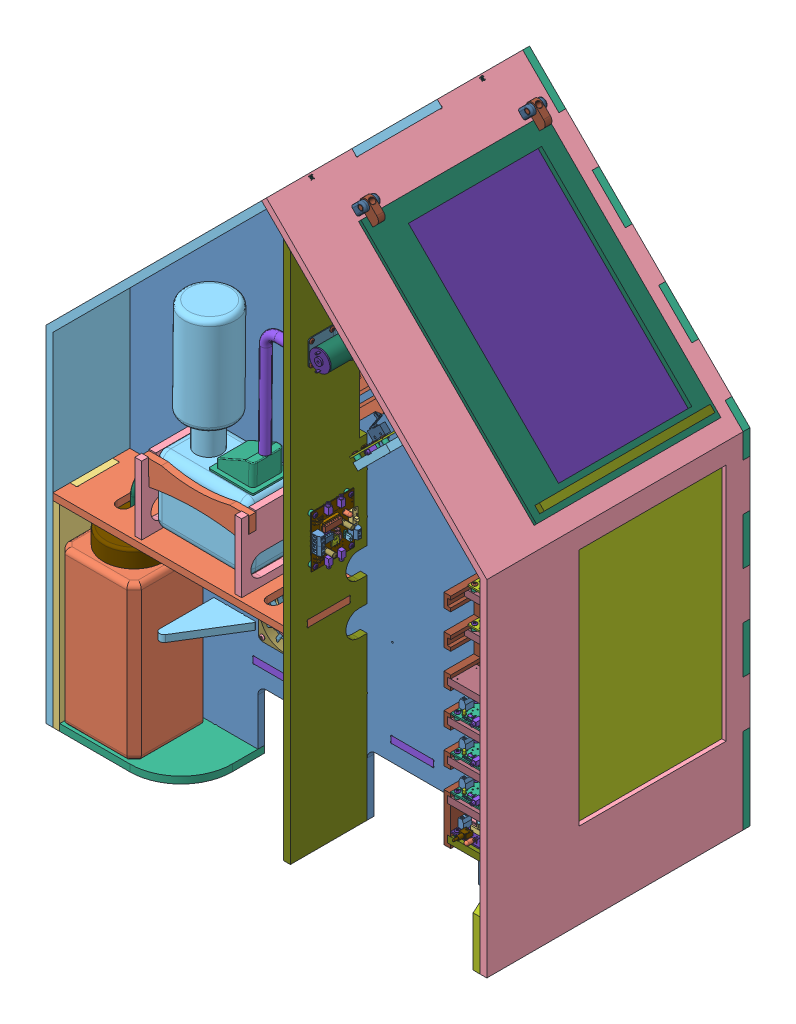
SolidWorks assembly Serre Toutes Options, configuration OLED. Lengths in mm. (continued)
Components (placement in the parent): (continued)
- VIS TORCX TF 3 X 19-50: VIS TORCX TF 3 X 19 [Défaut] at (178.8547 -145.9656 -4) x (-0.923728 -0.383049 0) z (0 0 -1)
- VIS TORCX TF 3 X 19-51: VIS TORCX TF 3 X 19 [Défaut] at (116.8547 -145.9656 -4) x (-0.923728 -0.383049 0) z (0 0 -1)
- VIS TORCX TF 3 X 19-52: VIS TORCX TF 3 X 19 [Défaut] at (178.8547 -7.9656 -4) x (-0.923728 -0.383049 0) z (0 0 -1)
- VIS TORCX TF 3 X 19-53: VIS TORCX TF 3 X 19 [Défaut] at (116.8547 -7.9656 -4) x (-0.923728 -0.383049 0) z (0 0 -1)
- Sous ensemble Arrosage-1: Sous ensemble Arrosage [Défaut] at (-248.1801 -261.6655 37.8651) x (-0.00308 0 0.999995) z (0 -1 0) size (140.54 240.54 274.35)
  - Pompe-1: Pompe [Défaut] at (-9.0938 -0.5877 17.5) size (40 29 55)
  - Tuyau gouteur-1: Tuyau gouteur [Défaut] at (-69.6171 -162.8404 -195.5) x (0 0 -1) z (0.999995 -0.00308 0) size (203 173 86)
  - Gouteur-1: Gouteur [Défaut] at (-70.8858 -170.9803 -151.85) x (-0.999995 0.00308 0) z (0 0 1) size (21 26.3 133.2)
    - PiedGouteur-1: PiedGouteur [Défaut] at (-1.2437 2.6563 -65) size (16 23.8 130)
    - BouchonGouteur-1: BouchonGouteur [Défaut] at (-1.2437 2.6563 -57) x (-0.923728 -0.383049 0) z (0 0 -1) size (16.07 16.07 11.2)
  - Bouchon reservoir-1: Bouchon reservoir [Défaut] at (10.9062 6.9123 -125.7) x (0.574699 -0.818365 0) z (0.818365 0.574699 0) size (71 20 71)
  - Passe cable-1: Passe cable [Défaut] at (10.9062 6.9123 -169.9434) x (0 0 -1) z (0 1 0) size (6 11 11)
  - Reservoir 1,25L-1: Reservoir 1,25L [Défaut] at (7.3532 24.2973 -125.7) x (0.999995 -0.00308 0) z (0 0 1) size (89.5 89.5 187)
- fondcuivré-1: fondcuivré [Défaut] at (-208.3657 -251.1382 -5)
- Capot complet-1: Capot complet [Vitres] at (-187.0166 -15.8593 -60) x (-1 0 0) z (0 0 -1) size (516 661.85 308)
  - Capot coté droit-1: Capot coté droit [Défaut] at (-332.1697 -265.6526 -154) size (263.66 661.85 308)
  - Capot coté gauche-1: Capot coté gauche [Défaut] at (175.8303 -266.1888 -154) size (263.66 661.85 308)
  - Capotfaçade-1: Capotfaçade [Défaut] at (75.9652 -264.3201 154) x (-1 0 0) z (0 0 -1) size (516 661.85 8)
  - Vitre laterale-1: Vitre laterale [Défaut] at (-385.1406 -165.6883 102.4285) x (0 1 0) z (1 0 0) size (290.43 181.9 2)
  - Vitre avant grande-1: Vitre avant grande [Défaut] at (-355.6546 -169.3327 147) x (0 1 0) z (0 0 1) size (286.8 171.11 2)
  - Vitre laterale-2: Vitre laterale [Défaut] at (120.8594 30.4421 102.4285) x (0 -1 0) z (-1 0 0) size (290.43 181.9 2)
  - Vitre avant grande-2: Vitre avant grande [Défaut] at (-40.8684 -169.3327 147) x (0 1 0) z (0 0 1) size (286.8 171.11 2)
  - Vitre avant centrale-1: Vitre avant centrale [Défaut] at (-154.2178 43.2096 147) size (123.47 286.8 2)
  - Vitre laterale-4: Vitre laterale [Défaut] at (-65.085 276.7887 -22.3285) x (0.707107 -0.707107 0) z (0.707107 0.707107 0) size (290.43 181.9 2)
  - Charnière percée-1: Charnière percée [Défaut] at (-176.8635 321.0541 -74.2825) x (-0.707107 -0.707107 0) z (0 0 -1) size (25.5 17 19)
    - Charnière percée-1: Charnière percée [Défaut] at (-8.739 -12.0088 -9.5) size (11 16 19)
    - Charnièere percée  2-1: Charnièere percée  2 [Défaut] at (-8.739 1.9912 -4) size (25.5 13 19)
  - Charnière percée-2: Charnière percée [Défaut] at (-176.8635 321.0541 120.9123) x (-0.707107 -0.707107 0) z (0 0 -1) size (25.5 17 19)
    - Charnière percée-1: Charnière percée [Défaut] at (-8.739 -12.0088 -9.5) size (11 16 19)
    - Charnièere percée  2-1: Charnièere percée  2 [Défaut] at (-8.739 1.9912 -4) size (25.5 13 19)
  - VIS TORCX TF 3 X 13-4: VIS TORCX TF 3 X 13 [Défaut] at (-159.0106 315.56 -74.2825) x (0.5 0.5 -0.707107) z (0.707107 -0.707107 0) size (5.6 5.6 13)
  - VIS TORCX TF 3 X 13-5: VIS TORCX TF 3 X 13 [Défaut] at (-159.0106 315.56 120.9123) x (0.5 0.5 -0.707107) z (0.707107 -0.707107 0) size (5.6 5.6 13)
  - VIS TORCX TF 3 X 19-1: VIS TORCX TF 3 X 19 [Défaut] at (-386.1406 -283.1062 154)
  - VIS TORCX TF 3 X 19-2: VIS TORCX TF 3 X 19 [Défaut] at (-386.1406 -233.1062 154)
  - VIS TORCX TF 3 X 19-3: VIS TORCX TF 3 X 19 [Défaut] at (-386.1406 -125.6062 154)
  - VIS TORCX TF 3 X 19-4: VIS TORCX TF 3 X 19 [Défaut] at (-386.1406 -15.6062 154)
  - VIS TORCX TF 3 X 19-5: VIS TORCX TF 3 X 19 [Défaut] at (-386.1406 81.3179 154)
  - VIS TORCX TF 3 X 19-6: VIS TORCX TF 3 X 19 [Défaut] at (-376.7525 103.4731 154)
  - VIS TORCX TF 3 X 19-7: VIS TORCX TF 3 X 19 [Défaut] at (-307.8566 172.3691 154)
  - VIS TORCX TF 3 X 19-8: VIS TORCX TF 3 X 19 [Défaut] at (-230.0748 250.1508 154)
  - VIS TORCX TF 3 X 19-9: VIS TORCX TF 3 X 19 [Défaut] at (-150.5253 329.7003 154)
  - VIS TORCX TF 3 X 19-10: VIS TORCX TF 3 X 19 [Défaut] at (-134.969 350.9153 96) x (0.5 0.5 0.707107) z (-0.707107 0.707107 0)
  - VIS TORCX TF 3 X 19-11: VIS TORCX TF 3 X 19 [Défaut] at (-129.3121 350.9153 -4) x (0.5 -0.5 -0.707107) z (0.707107 0.707107 0)
  - VIS TORCX TF 3 X 19-22: VIS TORCX TF 3 X 19 [Défaut] at (-134.969 350.9153 -104) x (0.5 0.5 0.707107) z (-0.707107 0.707107 0)
  - VIS TORCX TF 3 X 19-24: VIS TORCX TF 3 X 19 [Défaut] at (-113.7558 329.7003 154)
  - VIS TORCX TF 3 X 19-25: VIS TORCX TF 3 X 19 [Défaut] at (-34.2063 250.1508 154)
  - VIS TORCX TF 3 X 19-26: VIS TORCX TF 3 X 19 [Défaut] at (43.5755 172.3691 154)
  - VIS TORCX TF 3 X 19-27: VIS TORCX TF 3 X 19 [Défaut] at (112.4714 103.4731 154)
  - VIS TORCX TF 3 X 19-28: VIS TORCX TF 3 X 19 [Défaut] at (121.8594 81.3179 154)
  - VIS TORCX TF 3 X 19-29: VIS TORCX TF 3 X 19 [Défaut] at (121.8594 -15.6062 154)
  - VIS TORCX TF 3 X 19-30: VIS TORCX TF 3 X 19 [Défaut] at (121.8594 -233.1062 154)
  - VIS TORCX TF 3 X 19-31: VIS TORCX TF 3 X 19 [Défaut] at (121.8594 -125.6062 154)
  - VIS TORCX TF 3 X 19-32: VIS TORCX TF 3 X 19 [Défaut] at (121.8594 -283.1062 154)
  - Aimant-1: Aimant [Défaut] at (122.8594 -288.1062 -134) x (0 0 1) z (-1 0 0) size (8 8 5)
  - Aimant-2: Aimant [Défaut] at (-387.1406 -288.1062 -134) x (0 0 -1) z (1 0 0) size (8 8 5)
  - VIS TF 2.2x6.4-114: VIS TF 2.2x6.4 [Défaut] at (-383.1406 75.3601 128.5) x (0 -1 0) z (1 0 0) size (4.2 4.2 6.4)
  - VIS TF 2.2x6.4-115: VIS TF 2.2x6.4 [Défaut] at (-383.1406 -67.3599 128.5) x (0 -1 0) z (1 0 0) size (4.2 4.2 6.4)
  - VIS TF 2.2x6.4-116: VIS TF 2.2x6.4 [Défaut] at (-383.1406 -210.0699 128.5) x (0 -1 0) z (1 0 0) size (4.2 4.2 6.4)
  - VIS TF 2.2x6.4-117: VIS TF 2.2x6.4 [Défaut] at (-383.2825 -210.0699 -48.4) x (0 -1 0) z (0 0 1) size (4.2 4.2 6.4)
  - VIS TF 2.2x6.4-118: VIS TF 2.2x6.4 [Défaut] at (-383.2825 -67.3599 -48.4) x (0 -1 0) z (0 0 1) size (4.2 4.2 6.4)
  - VIS TF 2.2x6.4-119: VIS TF 2.2x6.4 [Défaut] at (-383.2825 75.3601 -48.4) x (0 -1 0) z (0 0 1) size (4.2 4.2 6.4)
  - VIS TF 2.2x6.4-120: VIS TF 2.2x6.4 [Défaut] at (-372.6406 -210.6062 147) x (1 0 0) z (0 0 -1) size (4.2 4.2 6.4)
  - VIS TF 2.2x6.4-121: VIS TF 2.2x6.4 [Défaut] at (-206.5306 -210.6062 147) x (1 0 0) z (0 0 -1) size (4.2 4.2 6.4)
  - VIS TF 2.2x6.4-122: VIS TF 2.2x6.4 [Défaut] at (-191.4267 -210.6062 147) x (1 0 0) z (0 0 -1) size (4.2 4.2 6.4)
  - VIS TF 2.2x6.4-123: VIS TF 2.2x6.4 [Défaut] at (-72.9567 -210.6062 147) x (1 0 0) z (0 0 -1) size (4.2 4.2 6.4)
  - VIS TF 2.2x6.4-124: VIS TF 2.2x6.4 [Défaut] at (118.8594 -210.6062 128.5) x (0 1 0) z (-1 0 0) size (4.2 4.2 6.4)
  - VIS TF 2.2x6.4-125: VIS TF 2.2x6.4 [Défaut] at (-372.6406 -69.7062 147) x (1 0 0) z (0 0 -1) size (4.2 4.2 6.4)
  - VIS TF 2.2x6.4-126: VIS TF 2.2x6.4 [Défaut] at (-206.5306 -70.0886 147) x (1 0 0) z (0 0 -1) size (4.2 4.2 6.4)
  - VIS TF 2.2x6.4-127: VIS TF 2.2x6.4 [Défaut] at (-191.4267 -66.7062 147) x (1 0 0) z (0 0 -1) size (4.2 4.2 6.4)
  - VIS TF 2.2x6.4-128: VIS TF 2.2x6.4 [Défaut] at (-72.9567 -62.2592 147) x (1 0 0) z (0 0 -1) size (4.2 4.2 6.4)
  - VIS TF 2.2x6.4-129: VIS TF 2.2x6.4 [Défaut] at (118.8594 -67.8862 128.5) x (0 1 0) z (-1 0 0) size (4.2 4.2 6.4)
  - VIS TF 2.2x6.4-130: VIS TF 2.2x6.4 [Défaut] at (-372.6406 71.1938 147) x (-0.923728 -0.383049 0) z (0 0 -1) size (4.2 4.2 6.4)
  - VIS TF 2.2x6.4-131: VIS TF 2.2x6.4 [Défaut] at (-206.5306 71.1938 147) x (1 0 0) z (0 0 -1) size (4.2 4.2 6.4)
  - VIS TF 2.2x6.4-132: VIS TF 2.2x6.4 [Défaut] at (-191.4267 71.1938 147) x (-0.923728 -0.383049 0) z (0 0 -1) size (4.2 4.2 6.4)
  - VIS TF 2.2x6.4-133: VIS TF 2.2x6.4 [Défaut] at (-72.9567 71.1938 147) x (1 0 0) z (0 0 -1) size (4.2 4.2 6.4)
  - VIS TF 2.2x6.4-134: VIS TF 2.2x6.4 [Défaut] at (118.8594 74.8238 128.5) x (0 1 0) z (-1 0 0) size (4.2 4.2 6.4)
  - VIS TF 2.2x6.4-135: VIS TF 2.2x6.4 [Défaut] at (118.8594 74.8238 -48.4) x (0 1 0) z (-1 0 0) size (4.2 4.2 6.4)
  - VIS TF 2.2x6.4-136: VIS TF 2.2x6.4 [Défaut] at (118.8594 -67.8862 -48.4) x (0 1 0) z (-1 0 0) size (4.2 4.2 6.4)
  - VIS TF 2.2x6.4-137: VIS TF 2.2x6.4 [Défaut] at (118.8594 -210.6062 -48.4) x (0 1 0) z (-1 0 0) size (4.2 4.2 6.4)
  - VIS TF 2.2x6.4-138: VIS TF 2.2x6.4 [Défaut] at (-57.8544 -210.6062 147) x (1 0 0) z (0 0 -1) size (4.2 4.2 6.4)
  - VIS TF 2.2x6.4-139: VIS TF 2.2x6.4 [Défaut] at (108.2556 -210.6062 147) x (1 0 0) z (0 0 -1) size (4.2 4.2 6.4)
  - VIS TF 2.2x6.4-140: VIS TF 2.2x6.4 [Défaut] at (-57.8544 -69.7062 147) x (1 0 0) z (0 0 -1) size (4.2 4.2 6.4)
  - VIS TF 2.2x6.4-141: VIS TF 2.2x6.4 [Défaut] at (108.2556 -70.0886 147) x (1 0 0) z (0 0 -1) size (4.2 4.2 6.4)
  - VIS TF 2.2x6.4-142: VIS TF 2.2x6.4 [Défaut] at (-57.8544 71.1938 147) x (1 0 0) z (0 0 -1) size (4.2 4.2 6.4)
  - VIS TF 2.2x6.4-143: VIS TF 2.2x6.4 [Défaut] at (108.2556 71.1938 147) x (1 0 0) z (0 0 -1) size (4.2 4.2 6.4)
  - VIS TF 2.2x6.4-144: VIS TF 2.2x6.4 [Défaut] at (107.098 88.486 147) x (1 0 0) z (0 0 -1) size (4.2 4.2 6.4)
  - VIS TF 2.2x6.4-145: VIS TF 2.2x6.4 [Défaut] at (105.3619 106.3418 128.5) x (-0.707107 0.707107 0) z (-0.707107 -0.707107 0) size (4.2 4.2 6.4)
  - VIS TF 2.2x6.4-146: VIS TF 2.2x6.4 [Défaut] at (105.3619 106.3418 -48.4) x (-0.707107 0.707107 0) z (-0.707107 -0.707107 0) size (4.2 4.2 6.4)
  - VIS TF 2.2x6.4-147: VIS TF 2.2x6.4 [Défaut] at (-131.8128 86.5458 147) x (1 0 0) z (0 0 -1) size (4.2 4.2 6.4)
  - VIS TF 2.2x6.4-148: VIS TF 2.2x6.4 [Défaut] at (4.4436 207.2601 -48.4) x (-0.707107 0.707107 0) z (-0.707107 -0.707107 0) size (4.2 4.2 6.4)
  - VIS TF 2.2x6.4-149: VIS TF 2.2x6.4 [Défaut] at (-3.5291 201.728 147) x (1 0 0) z (0 0 -1) size (4.2 4.2 6.4)
  - VIS TF 2.2x6.4-150: VIS TF 2.2x6.4 [Défaut] at (-96.4676 308.1713 -48.4) x (-0.707107 0.707107 0) z (-0.707107 -0.707107 0) size (4.2 4.2 6.4)
  - VIS TF 2.2x6.4-151: VIS TF 2.2x6.4 [Défaut] at (-96.4676 308.1713 128.5) x (-0.707107 0.707107 0) z (-0.707107 -0.707107 0) size (4.2 4.2 6.4)
  - VIS TF 2.2x6.4-152: VIS TF 2.2x6.4 [Défaut] at (-131.8128 309.8158 147) x (1 0 0) z (0 0 -1) size (4.2 4.2 6.4)
  - VIS TF 2.2x6.4-153: VIS TF 2.2x6.4 [Défaut] at (4.4436 207.2601 128.5) x (-0.707107 0.707107 0) z (-0.707107 -0.707107 0) size (4.2 4.2 6.4)
  - VIS TF 2.2x6.4-154: VIS TF 2.2x6.4 [Défaut] at (-370.7236 88.486 147) x (1 0 0) z (0 0 -1) size (4.2 4.2 6.4)
  - VIS TF 2.2x6.4-155: VIS TF 2.2x6.4 [Défaut] at (-260.0965 201.728 147) x (1 0 0) z (0 0 -1) size (4.2 4.2 6.4)
  - Fenêtre complete-1: Fenêtre complete [Défaut] at (-268.7504 217.134 52.5771) x (0 0 1) z (-0.707107 0.707107 0) size (216 290.55 23)
    - Fenêtre-1: Fenêtre [Défaut] at (-151.0146 -563.7006 -4) size (216 290.55 8)
    - poignée fenetre-1: poignée fenetre [Défaut] at (-29.6647 -138.358 4) x (1 0 0) z (0 -1 0) size (200 15 8)
    - Vitre fenetre-1: Vitre fenetre [Défaut] at (-68.8332 -67.4201 -4) x (0 1 0) z (0 0 1) size (258.45 165.9 2)
    - VIS TF 2.2x6.4-15: VIS TF 2.2x6.4 [Défaut] at (60.7353 -134.7546 -4) x (-0.714663 -0.699469 0) z (0 0 -1) size (4.2 4.2 6.4)
    - VIS TF 2.2x6.4-16: VIS TF 2.2x6.4 [Défaut] at (60.7353 -8.0346 -4) x (-0.714663 -0.699469 0) z (0 0 -1) size (4.2 4.2 6.4)
    - VIS TF 2.2x6.4-17: VIS TF 2.2x6.4 [Défaut] at (60.7353 118.6954 -4) x (-0.714663 -0.699469 0) z (0 0 -1) size (4.2 4.2 6.4)
    - VIS TF 2.2x6.4-18: VIS TF 2.2x6.4 [Défaut] at (-100.1647 118.6954 -4) x (-0.714663 -0.699469 0) z (0 0 -1) size (4.2 4.2 6.4)
    - VIS TF 2.2x6.4-19: VIS TF 2.2x6.4 [Défaut] at (-100.1647 -8.0346 -4) x (-0.714663 -0.699469 0) z (0 0 -1) size (4.2 4.2 6.4)
    - VIS TF 2.2x6.4-20: VIS TF 2.2x6.4 [Défaut] at (-100.1647 -134.7546 -4) x (-0.714663 -0.699469 0) z (0 0 -1) size (4.2 4.2 6.4)
    - VIS TORCX TF 3 X 19-1: VIS TORCX TF 3 X 19 [Défaut] at (-101.3516 -142.358 -4) x (-0.923728 -0.383049 0) z (0 0 -1)
    - VIS TORCX TF 3 X 19-2: VIS TORCX TF 3 X 19 [Défaut] at (43.6484 -142.358 -4) x (-0.923728 -0.383049 0) z (0 0 -1)
  - VIS TORCX TF 3 X 13-1: VIS TORCX TF 3 X 13 [Défaut] at (-174.567 311.3174 120.9123) x (-0.355164 -0.355164 0.864706) z (0.707107 -0.707107 0) size (5.6 5.6 13)
  - VIS TORCX TF 3 X 13-2: VIS TORCX TF 3 X 13 [Défaut] at (-174.567 311.3174 -74.3702) x (-0.355164 -0.355164 0.864706) z (0.707107 -0.707107 0) size (5.6 5.6 13)
  - Vitre triangulaire-2: Vitre triangulaire [Défaut] at (-131.8128 83.7958 147) size (490.22 227.27 2)
- Cache Oled-2: Cache Oled [Défaut] at (-241.7989 -284.4707 -216)
- guillotine-1: guillotine [Défaut] at (-150.376 -16.7665 73.5)
- Sonde capteur humidité-1: Sonde capteur humidité [Défaut] at (349.3697 -143.9656 -111.3159) x (1 0 0) z (0 1 0) size (30.38 36.99 128)
  - Base capteur humidité terre-1: Base capteur humidité terre [Défaut] at (-210.4875 -4.2437 -4) size (29.6 36.6 12.37)
  - Capot capteur humidité terre-1: Capot capteur humidité terre [Défaut] at (-210.4875 -4.2437 32.3863) x (0 0 1) z (-0.999641 -0.026785 0) size (7 29.6 29.6)
  - Tige capteur humidité-1: Tige capteur humidité [Défaut] at (-221.4875 -4.2437 8) x (1 0 0) z (0 1 0) size (3 50 3)
  - Tige capteur humidité-2: Tige capteur humidité [Défaut] at (-199.4875 -4.2437 8) x (1 0 0) z (0 1 0) size (3 50 3)
  - CI capteur humidité terre-1: CI capteur humidité terre [Défaut] at (-210.4875 -4.2437 3) size (25.6 25.6 1.6)
  - Vis 2.2 x 9.5-1: Vis 2.2 x 9.5 [Défaut] at (-210.4875 -4.2437 9.6) x (0.624792 0.780791 0) z (0.780791 -0.624792 0) size (4.27 12.1 4.27)
  - Résistance 75 Kohm Pas de 10-1: Résistance 75 Kohm Pas de 10 [Défaut] at (-210.4875 -12.0088 0.7228) x (1 0 0) z (0 1 0) size (10.5 4.15 2.3)
- OLED 4 lignes-1: OLED 4 lignes [Branchement Ecran] at (-224.8149 -274.3119 -201.15) x (-1 0 0) z (0 0 -1) size (112.48 60 17.95)
  - OLED Ecran-1: OLED Ecran [Défaut] at (16.4619 -2.1442 -3.15) size (98 60 6.3)
  - OLED Carte-1: OLED Carte [Défaut] at (-30.3146 19.8208 -6.05) x (-1 0 0) z (0 0 -1) size (58.76 19.26 17.5)
    - OLED CI-1: OLED CI [Défaut] at (-27.8956 -10.4745 -0.75) size (56.5 19 1.5)
    - PICOT-1: PICOT [Default] at (2.3498 -15.5392 -2.9) size (2.51 2.51 10)
    - PICOT-2: PICOT [Default] at (-47.4203 24.0709 2.9) x (0 1 0) z (0 0 -1) size (2.51 2.51 10)
    - PICOT-3: PICOT [Default] at (-43.441 -32.0492 2.9) x (-1 0 0) z (0 0 -1) size (2.51 2.51 10)
    - PICOT-6: PICOT [Default] at (4.8898 -15.5392 -2.9) size (2.51 2.51 10)
    - PICOT-7: PICOT [Default] at (7.4298 -15.5392 -2.9) size (2.51 2.51 10)
    - PICOT-8: PICOT [Default] at (9.9698 -15.5392 -2.9) size (2.51 2.51 10)
    - PICOT-9: PICOT [Default] at (12.5098 -15.5392 -2.9) size (2.51 2.51 10)
    - PICOT-10: PICOT [Default] at (15.0498 -15.5392 -2.9) size (2.51 2.51 10)
    - PICOT-11: PICOT [Default] at (17.5898 -15.5392 -2.9) size (2.51 2.51 10)
    - PICOT-12: PICOT [Default] at (20.1298 -15.5392 -2.9) size (2.51 2.51 10)
    - PICOT-13: PICOT [Default] at (22.6698 -15.5392 -2.9) size (2.51 2.51 10)
    - PICOT-14: PICOT [Default] at (25.2098 -15.5392 -2.9) size (2.51 2.51 10)
    - PICOT-15: PICOT [Default] at (27.7498 -15.5392 -2.9) size (2.51 2.51 10)
    - PICOT-16: PICOT [Default] at (30.2898 -15.5392 -2.9) size (2.51 2.51 10)
    - PICOT-17: PICOT [Default] at (32.8298 -15.5392 -2.9) size (2.51 2.51 10)
    - PICOT-18: PICOT [Default] at (35.3698 -15.5392 -2.9) size (2.51 2.51 10)
    - PICOT-19: PICOT [Default] at (-47.4203 26.6109 2.9) x (0 1 0) z (0 0 -1) size (2.51 2.51 10)
    - PICOT-20: PICOT [Default] at (-47.4203 29.1509 2.9) x (0 1 0) z (0 0 -1) size (2.51 2.51 10)
    - PICOT-21: PICOT [Default] at (-40.901 -32.0492 2.9) x (-1 0 0) z (0 0 -1) size (2.51 2.51 10)
    - PICOT-22: PICOT [Default] at (-38.361 -32.0492 2.9) x (-1 0 0) z (0 0 -1) size (2.51 2.51 10)
    - PICOT-23: PICOT [Default] at (-35.821 -32.0492 2.9) x (-1 0 0) z (0 0 -1) size (2.51 2.51 10)
    - PICOT-24: PICOT [Default] at (-33.281 -32.0492 2.9) x (-1 0 0) z (0 0 -1) size (2.51 2.51 10)
    - Résistance 10 K pas 10.16-1: Résistance 10 K pas 10.16 [Défaut] at (-21.8156 -8.9845 2.25) x (1 0 0) z (0 -1 0) size (10.66 4.15 2.3)
    - Résistance 10 K pas 10.16-2: Résistance 10 K pas 10.16 [Défaut] at (22.5244 -8.9845 2.25) x (1 0 0) z (0 -1 0) size (10.66 4.15 2.3)
    - Résistance 220 ohm pas 10.16-1: Résistance 220 ohm pas 10.16 [Défaut] at (3.5844 -8.9845 2.25) x (1 0 0) z (0 -1 0) size (10.66 4.15 2.3)
    - Support CI 18 pattes-1: Support CI 18 pattes [Défaut] at (4.7444 1.1755 0.75) x (-1 0 0) z (0 1 0) size (22.64 6 10.1)
    - CI 18 pattes-1: CI 18 pattes [Défaut] at (4.7444 1.1755 3.75) x (-1 0 0) z (0 1 0) size (22.64 7.2 7.8)
    - Embase program 3.5-1: Embase program 3.5 [Défaut] at (16.4044 -0.9745 0.75) x (0 -1 0) z (-1 0 0) size (12 8.56 14.2)
- Module Bouton poussoir K-AP-MBP-1: Module Bouton poussoir K-AP-MBP [Défaut] at (-164.8765 -275.7028 -194.7554) x (0 1 0) z (-1 0 0) size (32.91 17.91 54)
  - CI-AP-MLBP avec jack-1: CI-AP-MLBP avec jack [Défaut] at (1.1247 -1.2172 0) size (32.91 8.01 54)
    - CI BP et DEL-1: CI BP et DEL [Défaut] at (-14.8869 -1.2382 0) size (30 1.6 54)
    - Embase jack 2.5-1: Embase jack 2.5 [Défaut] at (-14.8868 -1.2382 -27.0002) x (1 0 0) z (0 0 -1) size (10.81 8.01 5)
  - Résistance 10 K pas 11-1: Résistance 10 K pas 11 [Défaut] at (-7.2623 0.5446 -37.4997) x (0 0 -1) z (1 0 0) size (11.5 4.15 2.3)
  - Bouton poussoir 12x12-1: Bouton poussoir 12x12 [Défaut] at (1.2433 -0.8554 -12.9124) x (0 0 -1) z (1 0 0) size (13.73 14.31 12.7)
- K-AP-MOLED-1: K-AP-MOLED [Défaut] at (-98.2989 -281.8003 -193.9) x (-1 0 0) z (0 0 1) size (32.91 54 33.12)
  - CI AP-EIR avec embase-1: CI AP-EIR avec embase [Défaut] at (-2.9015 -0.264 0) size (32.91 54 8.01)
    - CI AP-EIR-1: CI AP-EIR [Défaut] at (-19.5215 -26.5712 0) size (30 54 1.6)
    - Embase jack 2.5-1: Embase jack 2.5 [Défaut] at (-19.5215 0.429 1.6) x (1 0 0) z (0 -1 0) size (10.81 8.01 5)
  - ASB 3PICOTS-1: ASB 3PICOTS [Default] at (1.743 2.5589 5.703) x (0 1 0) z (0 0 -1) size (7.59 2.51 10)
    - PICOT-1: PICOT [Default] at (26.8516 -23.7306 1.953) size (2.51 2.51 10)
    - PICOT-2: PICOT [Default] at (29.3916 -23.7306 1.953) size (2.51 2.51 10)
    - PICOT-3: PICOT [Default] at (24.3116 -23.7306 1.953) size (2.51 2.51 10)
  - Résistance 1 ohm pas 11-1: Résistance 1 ohm pas 11 [Défaut] at (-7.4233 -23.3351 3) x (1 0 0) z (0 -1 0) size (11.5 4.15 2.3)
- Entretoise CI-3: Entretoise CI [Défaut] at (-160.876 -263.4656 -198) size (5.9 5.9 4.1)
- Entretoise CI-4: Entretoise CI [Défaut] at (-160.876 -285.4656 -198) size (5.9 5.9 4.1)
- Entretoise CI-5: Entretoise CI [Défaut] at (-114.876 -263.4656 -198) size (5.9 5.9 4.1)
- Entretoise CI-6: Entretoise CI [Défaut] at (-114.876 -285.4656 -198) size (5.9 5.9 4.1)
- Entretoise CI-7: Entretoise CI [Défaut] at (-101.8754 -258.9657 -198) size (5.9 5.9 4.1)
- Entretoise CI-8: Entretoise CI [Défaut] at (-101.8754 -304.9651 -198) size (5.9 5.9 4.1)
- Entretoise CI-9: Entretoise CI [Défaut] at (-79.8765 -258.9657 -198) size (5.9 5.9 4.1)
- Entretoise CI-10: Entretoise CI [Défaut] at (-79.8765 -304.9651 -198) size (5.9 5.9 4.1)
- VIs TC 3 x 9-1: VIs TC 3 x 9 [Défaut] at (-160.876 -263.4656 -198.7) x (1 0 0) z (0 -1 0) size (5.6 10.69 5.6)
- VIs TC 3 x 9-2: VIs TC 3 x 9 [Défaut] at (-160.876 -285.4645 -198.7) x (1 0 0) z (0 -1 0) size (5.6 10.69 5.6)
- VIs TC 3 x 9-3: VIs TC 3 x 9 [Défaut] at (-114.876 -263.4656 -198.7) x (1 0 0) z (0 -1 0) size (5.6 10.69 5.6)
- VIs TC 3 x 9-4: VIs TC 3 x 9 [Défaut] at (-114.8766 -285.4645 -198.7) x (1 0 0) z (0 -1 0) size (5.6 10.69 5.6)
- VIs TC 3 x 9-5: VIs TC 3 x 9 [Défaut] at (-101.8754 -258.9657 -198.7) x (1 0 0) z (0 -1 0) size (5.6 10.69 5.6)
- VIs TC 3 x 9-6: VIs TC 3 x 9 [Défaut] at (-79.8765 -258.9657 -198.7) x (1 0 0) z (0 -1 0) size (5.6 10.69 5.6)
- VIs TC 3 x 9-7: VIs TC 3 x 9 [Défaut] at (-101.8754 -304.9651 -198.7) x (1 0 0) z (0 -1 0) size (5.6 10.69 5.6)
- VIs TC 3 x 9-8: VIs TC 3 x 9 [Défaut] at (-79.8765 -304.9651 -198.7) x (1 0 0) z (0 -1 0) size (5.6 10.69 5.6)
- VIs TC 3 x 6.5-1: VIs TC 3 x 6.5 [Défaut] at (-273.876 -246.9656 -204.4) x (0.673476 -0.739209 0) z (-0.739209 -0.673476 0) size (5.6 8.09 5.6)
- VIs TC 3 x 6.5-2: VIs TC 3 x 6.5 [Défaut] at (-180.876 -301.9656 -204.4) x (0.673476 -0.739209 0) z (-0.739209 -0.673476 0) size (5.6 8.09 5.6)
- VIs TC 3 x 6.5-3: VIs TC 3 x 6.5 [Défaut] at (-273.876 -301.9656 -204.4) x (0.673476 -0.739209 0) z (-0.739209 -0.673476 0) size (5.6 8.09 5.6)
- Plateau chauffant-1: Plateau chauffant [Défaut] at (-58.8493 -230.9606 -113.4733) x (-1 0 0) z (0 -1 0) size (492 185 24.5)
  - Plateau chauffant desssous-1: Plateau chauffant desssous [Défaut] at (-179.8657 -72.1493 -4.995) size (492 185 10.01)
  - Plateau chauffant résistance-1: Plateau chauffant résistance [Défaut] at (-239.9733 76.0267 -2.495) x (1 0 0) z (0 1 0) size (477 22.5 165)
  - Plateau chauffant dessus-1: Plateau chauffant dessus [Défaut] at (-194.7641 -63.3329 -4.995) x (1 0 0) z (0 0 -1) size (492 185 2)
  - VIS TORCX TF 2.2X9.5-1: VIS TORCX TF 2.2X9.5 [Défaut] at (234.0267 80.5267 -6.995) x (-0.974823 -0.222981 0) z (0 0 -1) size (4.2 4.2 9.5)
  - VIS TORCX TF 2.2X9.5-2: VIS TORCX TF 2.2X9.5 [Défaut] at (234.0267 -88.4733 -6.995) x (-0.974823 -0.222981 0) z (0 0 -1) size (4.2 4.2 9.5)
  - VIS TORCX TF 2.2X9.5-3: VIS TORCX TF 2.2X9.5 [Défaut] at (-3.9733 -88.4733 -6.995) x (-0.974823 -0.222981 0) z (0 0 -1) size (4.2 4.2 9.5)
  - VIS TORCX TF 2.2X9.5-4: VIS TORCX TF 2.2X9.5 [Défaut] at (-3.9733 80.5267 -6.995) x (-0.974823 -0.222981 0) z (0 0 -1) size (4.2 4.2 9.5)
  - VIS TORCX TF 2.2X9.5-5: VIS TORCX TF 2.2X9.5 [Défaut] at (-241.9733 80.5267 -6.995) x (-0.974823 -0.222981 0) z (0 0 -1) size (4.2 4.2 9.5)
  - VIS TORCX TF 2.2X9.5-6: VIS TORCX TF 2.2X9.5 [Défaut] at (-241.9733 -88.4733 -6.995) x (-0.974823 -0.222981 0) z (0 0 -1) size (4.2 4.2 9.5)
- Sous ensemble Brumisateur complet-1: Sous ensemble Brumisateur complet [Défaut] at (-163.8767 30.3369 42.2196) x (-0.999957 0.009304 0) z (0.009304 0.999957 0) size (160 124.45 474.22)
  - volumebrumi-1: volumebrumi [Défaut] at (-31.9455 -18.4946 -115) size (110 68 230)
  - basebrumi-1: basebrumi [Défaut] at (-25.0537 -3.4946 -40) size (52 47 43.5)
  - picobrumisateurbis-1: picobrumisateurbis [Défaut] at (-106.4381 -34.2196 275.9424) x (1 0 0) z (0 -1 0) size (18 18.19 25.07)
  - Durite brumisateur-1: Durite brumisateur [Défaut] at (-50.9381 -4.7196 -7.0576) x (0 -1 0) z (-1 0 0) size (45 288.5 66.5)
Mates (geometry in assembly coordinates):
- Coïncidente1: coincident anti-aligned: axis of FONDINTERIEUR-1 through (57.939 191.6778 -4) axis (0 0 1); axis of Rondelle métal 3 x 12-1 through (57.939 191.6778 8.8) axis (0 0 -1)
- Coïncidente2: coincident anti-aligned: axis of Rondelle métal 3 x 12-1 through (57.939 191.6778 8.8) axis (0 0 -1); axis of VIs TC 3 x 13-1 through (57.939 191.6778 -1.7) axis (0 0 1)
- Coïncidente3: coincident anti-aligned: axis of FONDINTERIEUR-1 through (22.5836 156.3225 -4) axis (0 0 1); axis of Rondelle métal 3 x 12-2 through (22.5836 156.3225 8.8) axis (0 0 -1)
- Coïncidente4: coincident anti-aligned: axis of VIs TC 3 x 13-2 through (22.5836 156.3225 -1.7) axis (0 0 1); axis of Rondelle métal 3 x 12-2 through (22.5836 156.3225 8.8) axis (0 0 -1)
- Coïncidente5: coincident aligned: circle of VIs TC 3 x 13-2; plane of Rondelle métal 3 x 12-2 through (22.5836 156.3225 8.8) normal (0 0 1)
- Coïncidente6: coincident anti-aligned: plane of Rondelle métal 3 x 12-1 through (57.939 191.6778 8.8) normal (0 0 1); plane of VIs TC 3 x 13-1 through (57.939 191.6778 8.8) normal (0 0 -1)
- Coïncidente14: coincident anti-aligned: axis of FONDINTERIEUR-1 through (57.939 191.6778 -4) axis (0 0 1); axis of Entretoise CI-1 through (57.939 191.6778 8.1) axis (0 0 -1)
- Coïncidente15: coincident aligned: plane of FONDINTERIEUR-1 through (-297.9367 -225.0262 4) normal (0 0 1); circle of Entretoise CI-1
- Coïncidente16: coincident anti-aligned: axis of FONDINTERIEUR-1 through (22.5836 156.3225 -4) axis (0 0 1); axis of Entretoise CI-2 through (22.5836 156.3225 8.1) axis (0 0 -1)
- Coïncidente17: coincident aligned: plane of FONDINTERIEUR-1 through (-297.9367 -225.0262 4) normal (0 0 1); circle of Entretoise CI-2
- Tangent4: tangent anti-aligned: plane of Crémallière M3-3-1 through (-72.5742 65.3366 12) normal (0.707107 -0.707107 0); cylinder of Entretoise CI-2 through (22.5836 156.3225 8.1) axis (0 0 -1) radius 2.95
- Parallèle1: parallel aligned: plane of FONDINTERIEUR-1 through (-307.876 77.2771 4) normal (-0.707107 0.707107 0); plane of Crémallière M3-3-1 through (-52.7752 102.1062 12) normal (-0.707107 0.707107 0)
- Coïncidente19: coincident anti-aligned: plane of FONDINTERIEUR-1 through (-297.9367 -225.0262 4) normal (0 0 1); plane of Crémallière M3-3-1 through (65.6965 199.3646 4) normal (0 0 -1)
- Coïncidente20: coincident aligned: axis of FONDINTERIEUR-1 through (57.939 191.6778 -4) axis (0 0 1); axis of VIs TC 3 x 13-1 through (57.939 191.6778 -1.7) axis (0 0 1)
- Coïncidente21: coincident anti-aligned: plane of Crémallière M3-3-1 through (-70.4528 63.2153 8) normal (0 0 1); plane of Rondelle métal 3 x 12-1 through (57.939 191.6778 8) normal (0 0 -1)
- Coïncidente22: coincident anti-aligned: plane of Crémallière M3-3-1 through (-70.4528 63.2153 8) normal (0 0 1); plane of Rondelle métal 3 x 12-2 through (22.5836 156.3225 8) normal (0 0 -1)
- Coïncidente23: coincident anti-aligned: plane of FONDINTERIEUR-1 through (62.7794 136.4142 -4) normal (0.707107 -0.707107 0); plane of Prépa 06 module Microrupteur-1/support capteur-1 through (87.5711 161.2058 2.9393) normal (-0.707107 0.707107 0)
- Coïncidente24: coincident anti-aligned: plane of FONDINTERIEUR-1 through (96.8921 167.5269 -4) normal (-0.707107 -0.707107 0); plane of Prépa 06 module Microrupteur-1/support capteur-1 through (95.3921 169.0269 -4) normal (0.707107 0.707107 0)
- Coïncidente25: coincident aligned: plane of FONDINTERIEUR-1 through (-297.9367 -225.0262 -4) normal (0 0 -1); plane of Prépa 06 module Microrupteur-1/support capteur-1 through (95.3921 169.0269 -4) normal (0 0 -1)
- Coïncidente26: coincident anti-aligned: plane of FONDINTERIEUR-1 through (-7.9312 65.7035 -4) normal (0.707107 -0.707107 0); plane of Prépa 06 module Microrupteur-2/support capteur-1 through (16.8604 90.4952 2.9393) normal (-0.707107 0.707107 0)
- Coïncidente27: coincident anti-aligned: plane of FONDINTERIEUR-1 through (26.1815 96.8162 -4) normal (-0.707107 -0.707107 0); plane of Prépa 06 module Microrupteur-2/support capteur-1 through (24.6815 98.3162 -4) normal (0.707107 0.707107 0)
- Coïncidente28: coincident aligned: plane of FONDINTERIEUR-1 through (-297.9367 -225.0262 -4) normal (0 0 -1); plane of Prépa 06 module Microrupteur-2/support capteur-1 through (24.6815 98.3162 -4) normal (0 0 -1)
- Coïncidente29: coincident anti-aligned: axis of FONDINTERIEUR-1 through (-138.876 -138.9656 -4) axis (0 0 1); axis of Ventilateur-1/Cage ventilateur-1 through (-138.876 -138.9656 14.4) axis (0 0 -1)
- Coïncidente30: coincident anti-aligned: axis of FONDINTERIEUR-1 through (-88.876 -138.9656 -4) axis (0 0 1); axis of Ventilateur-1/Cage ventilateur-1 through (-88.876 -138.9656 14.4) axis (0 0 -1)
- Coïncidente31: coincident: plane of FONDINTERIEUR-1 through (-297.9367 -225.0262 4) normal (0 0 1); line of Ventilateur-1/Cage ventilateur-1 through (-143.876 -138.9656 4) axis (0 -1 0)
- Coïncidente32: coincident anti-aligned: axis of Ventilateur-1/Cage ventilateur-1 through (-138.876 -138.9656 14.4) axis (0 0 -1); axis of VIs TC 3 x 13-4 through (-138.876 -138.9656 3.9) axis (0 0 1)
- Coïncidente33: coincident anti-aligned: axis of Ventilateur-1/Cage ventilateur-1 through (-88.876 -138.9656 14.4) axis (0 0 -1); axis of VIs TC 3 x 13-6 through (-88.876 -138.9656 3.9) axis (0 0 1)
- Coïncidente34: coincident anti-aligned: axis of Ventilateur-1/Cage ventilateur-1 through (-88.876 -188.9656 14.4) axis (0 0 -1); axis of VIs TC 3 x 13-7 through (-88.876 -188.9656 3.9) axis (0 0 1)
- Coïncidente35: coincident anti-aligned: axis of Ventilateur-1/Cage ventilateur-1 through (-138.876 -188.9656 14.4) axis (0 0 -1); axis of VIs TC 3 x 13-8 through (-138.876 -188.9656 3.9) axis (0 0 1)
- Coïncidente36: coincident aligned: plane of Ventilateur-1/Cage ventilateur-1 through (-88.876 -138.9656 14.4) normal (0 0 1); circle of VIs TC 3 x 13-8
- Coïncidente37: coincident aligned: plane of Ventilateur-1/Cage ventilateur-1 through (-88.876 -138.9656 14.4) normal (0 0 1); circle of VIs TC 3 x 13-4
- Coïncidente38: coincident aligned: plane of Ventilateur-1/Cage ventilateur-1 through (-88.876 -138.9656 14.4) normal (0 0 1); circle of VIs TC 3 x 13-6
- Coïncidente39: coincident aligned: plane of Ventilateur-1/Cage ventilateur-1 through (-88.876 -138.9656 14.4) normal (0 0 1); circle of VIs TC 3 x 13-7
- Coïncidente40: coincident aligned: axis of FONDINTERIEUR-1 through (8.418 76.3959 4) axis (0 0 -1); axis of VIS TORCX TF 3 X 19-2 through (8.418 76.3959 12.4885) axis (0 0 -1)
- Coïncidente41: coincident aligned: plane of FONDINTERIEUR-1 through (-297.9367 -225.0262 -4) normal (0 0 -1); plane of VIS TORCX TF 3 X 19-2 through (7.3455 78.9824 -4) normal (0 0 -1)
- Coïncidente42: coincident aligned: axis of FONDINTERIEUR-1 through (79.1287 147.1066 4) axis (0 0 -1); axis of VIS TORCX TF 3 X 19-1 through (79.1287 147.1066 12.4885) axis (0 0 -1)
- Coïncidente43: coincident aligned: plane of FONDINTERIEUR-1 through (-297.9367 -225.0262 -4) normal (0 0 -1); plane of VIS TORCX TF 3 X 19-1 through (78.0561 149.693 -4) normal (0 0 -1)
- Coïncidente44: coincident anti-aligned: plane of FONDINTERIEUR-1 through (-26.876 223.1558 -4) normal (-1 0 0); plane of Prépa 02 renfort arrière-1/renfortarriere-1 through (-26.876 272.0951 2.9393) normal (1 0 0)
- Coïncidente45: coincident anti-aligned: plane of FONDINTERIEUR-1 through (-28.9973 271.0344 -4) normal (0 -1 0); plane of Prépa 02 renfort arrière-1/renfortarriere-1 through (-26.876 271.0344 -4) normal (0 1 0)
- Coïncidente46: coincident aligned: plane of FONDINTERIEUR-1 through (-297.9367 -225.0262 -4) normal (0 0 -1); plane of Prépa 02 renfort arrière-1/renfortarriere-1 through (-26.876 221.1086 -4) normal (0 0 -1)
- Coïncidente47: coincident anti-aligned: plane of FONDINTERIEUR-1 through (-56.9973 -85.9656 -4) normal (0 -1 0); plane of étagèrebrumi-1 through (-297.9367 -85.9656 72.872) normal (0 1 0)
- Coïncidente48: coincident anti-aligned: plane of FONDINTERIEUR-1 through (-54.876 -88.0869 -4) normal (-1 0 0); plane of étagèrebrumi-1 through (-54.876 -85.9656 1.8787) normal (1 0 0)
- Coïncidente49: coincident aligned: plane of FONDINTERIEUR-1 through (-297.9367 -225.0262 -4) normal (0 0 -1); plane of étagèrebrumi-1 through (-54.876 -85.9656 -4) normal (0 0 -1)
- Coïncidente50: coincident anti-aligned: axis of FONDINTERIEUR-1 through (-30.876 -315.9656 -4) axis (0 0 1); axis of VIS TORCX TF 3 X 19-3 through (-30.876 -315.9656 12.4885) axis (0 0 -1)
